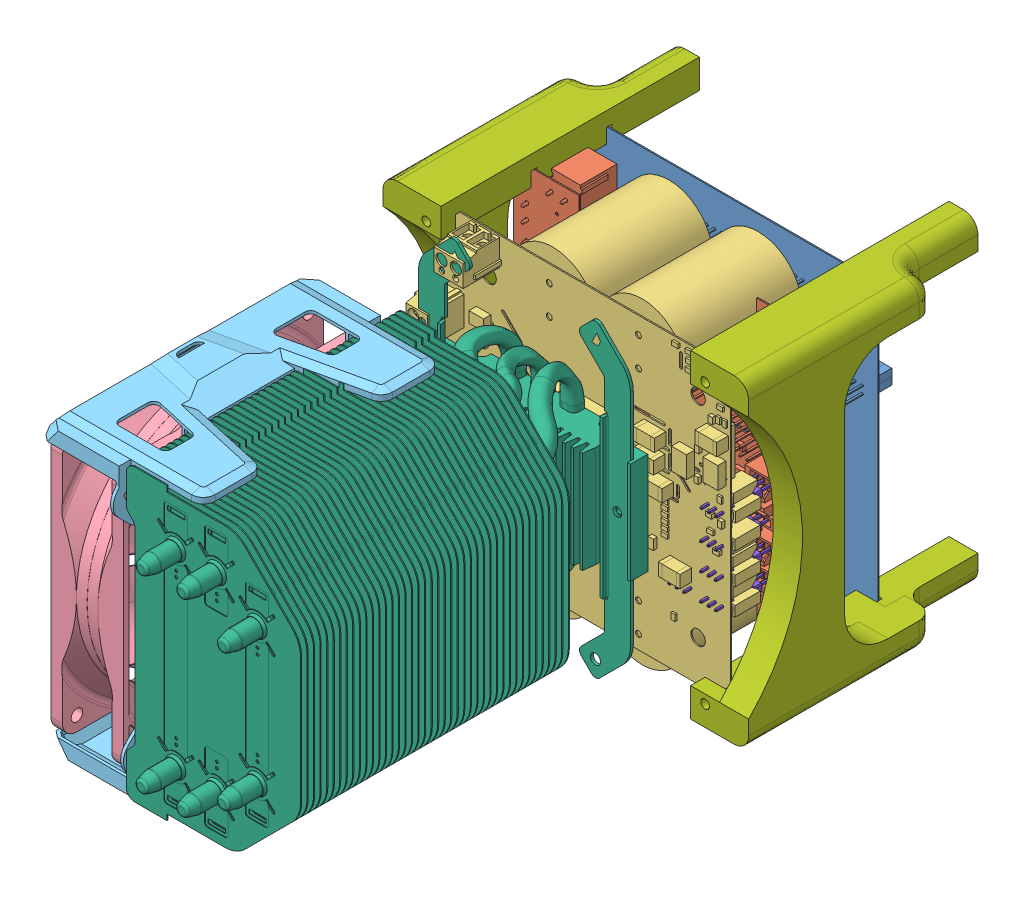
SolidWorks assembly REV3.0.1, configuration Default. Lengths in mm.
Overall size (190.84 111.69 228.07).
26 component instances, 9 part files, 61 mates.
Components (placement in the parent):
- controlo_rev3-1: controlo_rev3 [Default] at (-50.1858 -26.7845 -12.6892) size (100.07 100.84 29.54)
- middlePCB_rev3-1: middlePCB_rev3 [Default] at (-50.1858 -26.7845 12.7222) size (100.36 100.9 32.46)
- inversor_rev3-1: inversor_rev3 [Default] at (-50.1858 -26.7845 38.1337) size (100.35 109.25 56.47)
- dissipador-1: dissipador [Default] at (4.979 -21.2139 126.7824) x (0 1 0) z (0 0 1) size (108.44 180.01 139.76)
  - 7030025_PART_FAN STANDARD 90_MODEL.igs-1: 7030025_PART_FAN STANDARD 90_MODEL.igs [Default] at (0 45 -45) x (1 0 0) z (0 -1 0) size (93.98 180.01 25.07)
  - 7030026_PART_HEATSINK ADAPTOR 90_MODEL.igs-1: 7030026_PART_HEATSINK ADAPTOR 90_MODEL.igs [Default] at (95 58.5 47.4641) x (0 0 -1) z (-1 0 0) size (106.39 52.6 26.58)
  - 7030026_PART_HEATSINK ADAPTOR 90_MODEL.igs-2: 7030026_PART_HEATSINK ADAPTOR 90_MODEL.igs [Default] at (-7 58.5 -46) x (0 0 1) z (1 0 0) size (106.39 52.6 26.58)
  - 7030027_PART_CPU HEATSINK TOWER_MODEL.igs-1: 7030027_PART_CPU HEATSINK TOWER_MODEL.igs [Default] at (94 31.5 -47.65) x (-1 0 0) z (0 0 1) size (108.44 80.01 139.76)
- suporte_conversor_rev31-1: suporte_conversor_rev31 [Default] at (-45.1858 21.2155 12.7222) x (0 -1 0) z (-1 0 0) size (110 89 20)
- suporte_conversor_rev31-2: suporte_conversor_rev31 [Default] at (40.8142 21.2155 12.7222) x (0 1 0) z (1 0 0) size (110 89 20)
- header_3p_dual-1: header_3p_dual [Default] at (-30.5008 0.4189 26.9672) x (1 0 0) z (0 1 0) size (7.56 24.1 2.51)
- header_3p_dual-2: header_3p_dual [Default] at (-30.5008 19.7102 26.9672) x (1 0 0) z (0 1 0) size (7.56 24.1 2.51)
- header_3p_dual-3: header_3p_dual [Default] at (-30.5008 39.0015 26.9672) x (1 0 0) z (0 1 0) size (7.56 24.1 2.51)
- header_3p_socket-1: header_3p_socket [Default] at (-30.5007 39.0015 12.7222) x (1 0 0) z (0 -1 0) size (7.62 19.78 2.54)
- header_3p_socket-2: header_3p_socket [Default] at (-30.5007 19.7102 12.7222) x (1 0 0) z (0 -1 0) size (7.62 19.78 2.54)
- header_3p_socket-3: header_3p_socket [Default] at (-30.5007 0.4189 12.7222) x (1 0 0) z (0 -1 0) size (7.62 19.78 2.54)
- header_3p_socket-4: header_3p_socket [Default] at (38.0793 -1.2575 12.7222) x (1 0 0) z (0 -1 0) size (7.62 19.78 2.54)
- header_3p_socket-5: header_3p_socket [Default] at (49.0012 -1.2575 12.7222) x (1 0 0) z (0 -1 0) size (7.62 19.78 2.54)
- header_3p_socket-6: header_3p_socket [Default] at (49.0012 7.7699 12.7222) x (1 0 0) z (0 -1 0) size (7.62 19.78 2.54)
- header_3p_socket-7: header_3p_socket [Default] at (49.0011 16.7765 12.7222) x (1 0 0) z (0 -1 0) size (7.62 19.78 2.54)
- header_3p_socket-8: header_3p_socket [Default] at (49.1536 26.8095 12.7222) x (1 0 0) z (0 -1 0) size (7.62 19.78 2.54)
- header_3p_dual-4: header_3p_dual [Default] at (38.0792 -1.2575 26.9672) x (1 0 0) z (0 1 0) size (7.56 24.1 2.51)
- header_3p_dual-5: header_3p_dual [Default] at (49.0011 7.77 26.9672) x (1 0 0) z (0 1 0) size (7.56 24.1 2.51)
- header_3p_dual-6: header_3p_dual [Default] at (49.0012 16.7765 26.9672) x (1 0 0) z (0 1 0) size (7.56 24.1 2.51)
- header_3p_dual-7: header_3p_dual [Default] at (49.1536 26.8095 26.9672) x (1 0 0) z (0 1 0) size (7.56 24.1 2.51)
- header_3p_dual-8: header_3p_dual [Default] at (49.0011 -1.2575 26.9672) x (1 0 0) z (0 1 0) size (7.56 24.1 2.51)
Mates (geometry in assembly coordinates):
- Concentric1: concentric: cylinder of middlePCB_rev3-1 through (-50.1858 69.2155 12.3108) axis (0 0 -1) radius 1.5; cylinder of inversor_rev3-1 through (-50.1858 69.2155 37.7222) axis (0 0 -1) radius 1.5
- Concentric2: concentric: cylinder of controlo_rev3-1 through (-50.1858 69.2155 -13.1007) axis (0 0 -1) radius 1.5; cylinder of middlePCB_rev3-1 through (-50.1858 69.2155 12.3108) axis (0 0 -1) radius 1.5
- Concentric3: concentric: cylinder of middlePCB_rev3-1 through (45.8142 69.2155 12.3108) axis (0 0 -1) radius 1.5; cylinder of inversor_rev3-1 through (45.8142 69.2155 37.7222) axis (0 0 -1) radius 1.5
- Concentric4: concentric: cylinder of controlo_rev3-1 through (45.8142 69.2155 -13.1007) axis (0 0 -1) radius 1.5; cylinder of middlePCB_rev3-1 through (45.8142 69.2155 12.3108) axis (0 0 -1) radius 1.5
- Distance1: distance = 25 mm: plane of middlePCB_rev3-1 through (-52.0908 -28.7895 12.7222) normal (0 0 1); plane of inversor_rev3-1 through (-52.1858 -28.6895 37.7222) normal (0 0 -1)
- Distance2: distance = 25 mm: plane of middlePCB_rev3-1 through (-52.0908 -28.7895 12.3108) normal (0 0 -1); plane of controlo_rev3-1 through (-52.1858 -28.6895 -12.6892) normal (0 0 1)
- Tangent2: tangent: plane of inversor_rev3-1 through (-3.8278 39.0361 44.1324) normal (0 0 1); face of dissipador-1/7030027_PART_CPU HEATSINK TOWER_MODEL.igs-1
- Tangent5: tangent: plane of inversor_rev3-1 through (-2.0778 40.2861 44.1324) normal (0 1 0); face of dissipador-1/7030027_PART_CPU HEATSINK TOWER_MODEL.igs-1
- Concentric5: concentric: cylinder of inversor_rev3-1 through (-50.1858 69.2155 37.7222) axis (0 0 -1) radius 1.5; cylinder of suporte_conversor_rev31-1 through (-50.1858 69.2155 -12.2778) axis (0 0 1) radius 1.5
- Concentric6: concentric: cylinder of inversor_rev3-1 through (-50.1858 -26.7845 37.7222) axis (0 0 -1) radius 1.5; cylinder of suporte_conversor_rev31-1 through (-50.1858 -26.7845 48.9649) axis (0 0 -1) radius 1.5
- Coincident1: coincident: plane of inversor_rev3-1 through (-52.1858 -28.6895 37.7222) normal (0 0 -1); plane of suporte_conversor_rev31-1 through (-55.1858 21.2155 37.7222) normal (0 0 1)
- Coincident2: coincident: cylinder of inversor_rev3-1 through (45.8142 -26.7845 37.7222) axis (0 0 -1) radius 1.5; circle of suporte_conversor_rev31-2
- Coincident3: coincident: plane of inversor_rev3-1 through (-52.1858 -28.6895 37.7222) normal (0 0 -1); plane of suporte_conversor_rev31-2 through (50.8142 21.2155 37.7222) normal (0 0 1)
- Concentric9: concentric: cylinder of inversor_rev3-1 through (-39.3908 0.4189 37.7222) axis (0 0 -1) radius 0.45; cylinder of header_3p_dual-1 through (-39.3908 0.4189 40.8222) axis (0 0 -1) radius 0.17
- Concentric10: concentric: cylinder of inversor_rev3-1 through (-34.3108 0.4189 37.7222) axis (0 0 -1) radius 0.45; cylinder of header_3p_dual-1 through (-34.3108 0.4189 40.8222) axis (0 0 -1) radius 0.17
- Coincident7: coincident: plane of inversor_rev3-1 through (-52.1858 -28.6895 37.7222) normal (0 0 -1); line of header_3p_dual-1 through (-40.6608 -0.3811 37.7222) axis (1 0 0)
- Concentric11: concentric: cylinder of inversor_rev3-1 through (-39.3908 19.7102 37.7222) axis (0 0 -1) radius 0.45; cylinder of header_3p_dual-2 through (-39.3908 19.7102 40.8222) axis (0 0 -1) radius 0.17
- Concentric12: concentric: cylinder of inversor_rev3-1 through (-34.3108 19.7102 37.7222) axis (0 0 -1) radius 0.45; cylinder of header_3p_dual-2 through (-34.3108 19.7102 40.8222) axis (0 0 -1) radius 0.17
- Coincident8: coincident: plane of inversor_rev3-1 through (-52.1858 -28.6895 37.7222) normal (0 0 -1); line of header_3p_dual-2 through (-40.3108 20.9652 37.7222) axis (1 0 0)
- Concentric13: concentric: cylinder of inversor_rev3-1 through (-36.8508 39.0015 37.7222) axis (0 0 -1) radius 0.45; cylinder of header_3p_dual-3 through (-36.8508 39.0015 40.8222) axis (0 0 -1) radius 0.17
- Concentric14: concentric: cylinder of inversor_rev3-1 through (-39.3908 39.0015 37.7222) axis (0 0 -1) radius 0.45; cylinder of header_3p_dual-3 through (-39.3908 39.0015 40.8222) axis (0 0 -1) radius 0.17
- Coincident9: coincident: plane of inversor_rev3-1 through (-52.1858 -28.6895 37.7222) normal (0 0 -1); line of header_3p_dual-3 through (-40.3108 40.2565 37.7222) axis (1 0 0)
- Concentric15: concentric: cylinder of middlePCB_rev3-1 through (-39.3907 39.0015 12.3108) axis (0 0 -1) radius 0.45; cylinder of header_3p_socket-1 through (-39.3907 39.0015 19.7222) axis (0 0 -1) radius 0.46
- Concentric16: concentric: cylinder of middlePCB_rev3-1 through (-36.8507 39.0015 12.3108) axis (0 0 -1) radius 0.45; cylinder of header_3p_socket-1 through (-36.8507 39.0015 19.7222) axis (0 0 -1) radius 0.46
- Coincident10: coincident: plane of middlePCB_rev3-1 through (-52.0908 -28.7895 12.7222) normal (0 0 1); plane of header_3p_socket-1 through (-39.4407 36.3892 12.7222) normal (0 0 -1)
- Concentric17: concentric: cylinder of middlePCB_rev3-1 through (-39.3907 19.7102 12.3108) axis (0 0 -1) radius 0.45; cylinder of header_3p_socket-2 through (-39.3907 19.7102 19.7222) axis (0 0 -1) radius 0.46
- Concentric18: concentric: cylinder of middlePCB_rev3-1 through (-36.8507 19.7102 12.3108) axis (0 0 -1) radius 0.45; cylinder of header_3p_socket-2 through (-36.8507 19.7102 19.7222) axis (0 0 -1) radius 0.46
- Coincident11: coincident: plane of middlePCB_rev3-1 through (-52.0908 -28.7895 12.7222) normal (0 0 1); line of header_3p_socket-2 through (-40.3806 20.9802 12.7222) axis (1 0 0)
- Concentric19: concentric: cylinder of middlePCB_rev3-1 through (-39.3907 0.4189 12.3108) axis (0 0 -1) radius 0.45; cylinder of header_3p_socket-3 through (-39.3907 0.4189 19.7222) axis (0 0 -1) radius 0.46
- Concentric20: concentric: cylinder of middlePCB_rev3-1 through (-36.8507 0.4189 12.3108) axis (0 0 -1) radius 0.45; cylinder of header_3p_socket-3 through (-36.8507 0.4189 19.7222) axis (0 0 -1) radius 0.46
- Coincident12: coincident: plane of middlePCB_rev3-1 through (-52.0908 -28.7895 12.7222) normal (0 0 1); line of header_3p_socket-3 through (-37.7406 1.6889 12.7222) axis (1 0 0)
- Concentric21: concentric: circle of middlePCB_rev3-1; cylinder of header_3p_socket-4 through (34.2693 -1.2575 19.7222) axis (0 0 -1) radius 0.46
- Concentric22: concentric: circle of middlePCB_rev3-1; cylinder of header_3p_socket-4 through (31.7293 -1.2575 19.7222) axis (0 0 -1) radius 0.46
- Coincident13: coincident: plane of middlePCB_rev3-1 through (-52.0908 -28.7895 12.7222) normal (0 0 1); point of header_3p_socket-4
- Concentric23: concentric: circle of middlePCB_rev3-1; cylinder of header_3p_socket-5 through (45.1912 -1.2575 19.7222) axis (0 0 -1) radius 0.46
- Concentric24: concentric: circle of middlePCB_rev3-1; cylinder of header_3p_socket-5 through (42.6512 -1.2575 19.7222) axis (0 0 -1) radius 0.46
- Coincident15: coincident: plane of middlePCB_rev3-1 through (-52.0908 -28.7895 12.7222) normal (0 0 1); line of header_3p_socket-5 through (46.0811 -2.5275 12.7222) axis (-1 0 0)
- Concentric25: concentric: cylinder of middlePCB_rev3-1 through (45.1912 7.7699 12.3108) axis (0 0 -1) radius 0.45; cylinder of header_3p_socket-6 through (45.1912 7.7699 19.7222) axis (0 0 -1) radius 0.46
- Concentric26: concentric: circle of middlePCB_rev3-1; cylinder of header_3p_socket-7 through (45.1911 16.7765 19.7222) axis (0 0 -1) radius 0.46
- Concentric27: concentric: cylinder of middlePCB_rev3-1 through (45.3436 26.8095 12.3108) axis (0 0 -1) radius 0.45; cylinder of header_3p_socket-8 through (45.3436 26.8095 19.7222) axis (0 0 -1) radius 0.46
- Concentric28: concentric: circle of middlePCB_rev3-1; cylinder of header_3p_socket-8 through (42.8036 26.8095 19.7222) axis (0 0 -1) radius 0.46
- Concentric29: concentric: circle of middlePCB_rev3-1; cylinder of header_3p_socket-7 through (42.6511 16.7765 19.7222) axis (0 0 -1) radius 0.46
- Concentric30: concentric: circle of middlePCB_rev3-1; cylinder of header_3p_socket-6 through (42.6512 7.7699 19.7222) axis (0 0 -1) radius 0.46
- Coincident16: coincident: plane of middlePCB_rev3-1 through (-52.0908 -28.7895 12.7222) normal (0 0 1); line of header_3p_socket-6 through (46.0811 6.4999 12.7222) axis (-1 0 0)
- Coincident17: coincident: plane of middlePCB_rev3-1 through (-52.0908 -28.7895 12.7222) normal (0 0 1); line of header_3p_socket-7 through (46.081 15.5065 12.7222) axis (-1 0 0)
- Coincident18: coincident: plane of middlePCB_rev3-1 through (-52.0908 -28.7895 12.7222) normal (0 0 1); line of header_3p_socket-8 through (46.2335 25.5395 12.7222) axis (-1 0 0)
- Concentric31: concentric: circle of inversor_rev3-1; cylinder of header_3p_dual-4 through (29.1892 -1.2575 40.8222) axis (0 0 -1) radius 0.17
- Concentric32: concentric: circle of inversor_rev3-1; cylinder of header_3p_dual-4 through (34.2692 -1.2575 40.8222) axis (0 0 -1) radius 0.17
- Coincident19: coincident: plane of inversor_rev3-1 through (-52.1858 -28.6895 37.7222) normal (0 0 -1); line of header_3p_dual-4 through (33.3492 -2.5125 37.7222) axis (1 0 0)
- Concentric33: concentric: circle of inversor_rev3-1; cylinder of header_3p_dual-8 through (40.1111 -1.2575 40.8222) axis (0 0 -1) radius 0.17
- Concentric34: concentric: circle of inversor_rev3-1; cylinder of header_3p_dual-8 through (42.6511 -1.2575 40.8222) axis (0 0 -1) radius 0.17
- Coincident20: coincident: plane of inversor_rev3-1 through (-52.1858 -28.6895 37.7222) normal (0 0 -1); line of header_3p_dual-8 through (44.2711 -2.5125 37.7222) axis (1 0 0)
- Concentric35: concentric: circle of inversor_rev3-1; cylinder of header_3p_dual-5 through (45.1911 7.77 40.8222) axis (0 0 -1) radius 0.17
- Concentric36: concentric: circle of inversor_rev3-1; cylinder of header_3p_dual-5 through (42.6511 7.77 40.8222) axis (0 0 -1) radius 0.17
- Coincident21: coincident: plane of inversor_rev3-1 through (-52.1858 -28.6895 37.7222) normal (0 0 -1); line of header_3p_dual-5 through (46.4011 8.625 37.7222) axis (-0.586968 0.80961 0)
- Concentric37: concentric: circle of inversor_rev3-1; cylinder of header_3p_dual-7 through (45.3436 26.8095 40.8222) axis (0 0 -1) radius 0.17
- Concentric38: concentric: circle of inversor_rev3-1; cylinder of header_3p_dual-7 through (42.8036 26.8095 40.8222) axis (0 0 -1) radius 0.17
- Coincident22: coincident: plane of inversor_rev3-1 through (-52.1858 -28.6895 37.7222) normal (0 0 -1); plane of header_3p_dual-7 through (38.9936 25.5545 37.7222) normal (0 0 1)
- Concentric39: concentric: circle of inversor_rev3-1; cylinder of header_3p_dual-6 through (45.1912 16.7765 40.8222) axis (0 0 -1) radius 0.17
- Concentric40: concentric: circle of inversor_rev3-1; cylinder of header_3p_dual-6 through (42.6512 16.7765 40.8222) axis (0 0 -1) radius 0.17
- Coincident23: coincident: plane of inversor_rev3-1 through (-52.1858 -28.6895 37.7222) normal (0 0 -1); plane of header_3p_dual-6 through (38.8412 15.5215 37.7222) normal (0 0 1)
